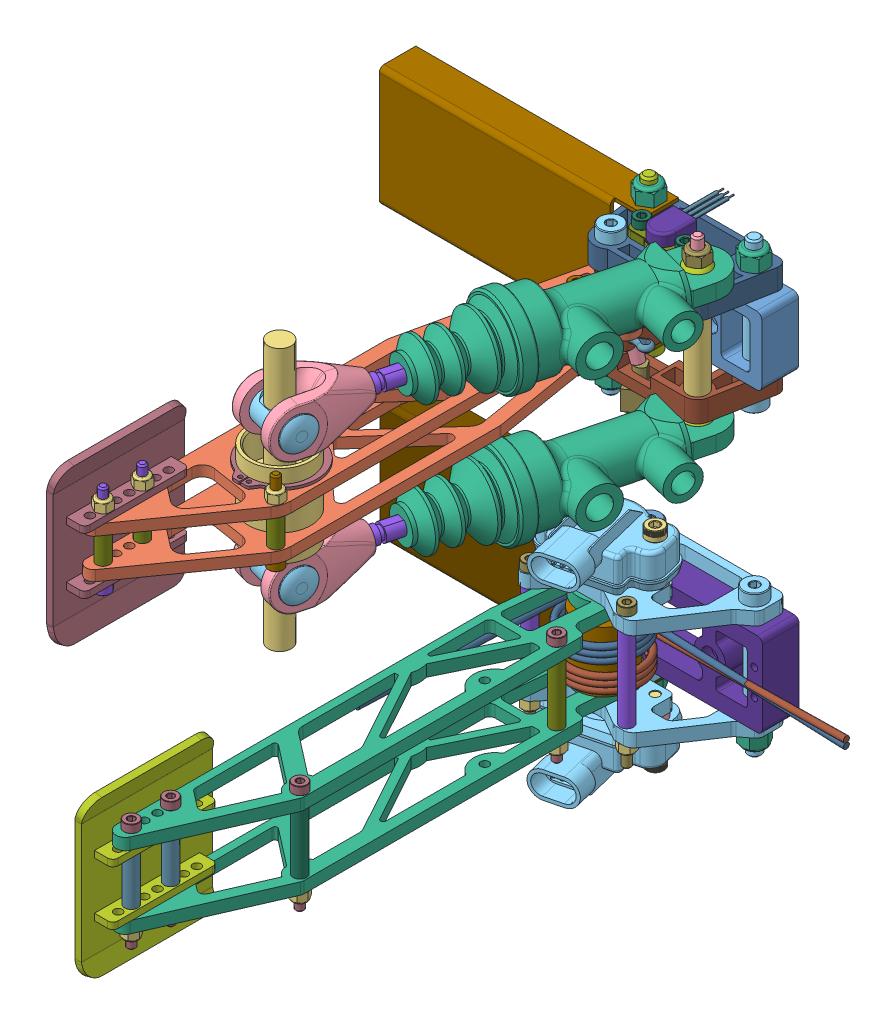
SolidWorks assembly BR-A10001-BC-Pedal Box Assembly, configuration Default. Lengths in mm.
Overall size (234.39 254.99 284.61).
117 component instances, 60 part files, 3 mates.
Components (placement in the parent):
- BR-10001-DC-Brake Pedal Assembly-1: BR-10001-DC-Brake Pedal Assembly [Default] at (189.4552 74.6925 66.1604) size (203.2 127 284.61)
  - BR-X000X-BC-Brake Pedal Platform-1: BR-X000X-BC-Brake Pedal Platform [Default] at (101.6 16.51 0) size (203.2 33.02 17.78)
  - BR-20002-AG-Brake Pedal Arm-3: BR-20002-AG-Brake Pedal Arm [Topo] at (131.445 12.065 13.97) size (50.8 6.35 239.54)
  - BR-20002-AG-Brake Pedal Arm-4: BR-20002-AG-Brake Pedal Arm [Topo] at (131.445 -6.985 13.97) size (50.8 6.35 239.54)
  - BR-00005-AA-Balance Bar (Tilton 600 Series)-1: BR-00005-AA-Balance Bar (Tilton 600 Series) [Default] at (131.445 0 174.2165) x (0.970657 0 0.240469) z (-0.240469 0 0.970657) size (31.09 127 49.61)
    - Copy of Bar^BR-00005-AA-Balance Bar (Tilton 600 Series)-1: Copy of Bar^BR-00005-AA-Balance Bar (Tilton 600 Series) [Default] at origin size (30.18 127 30.18) (virtual)
    - BB Arm^BR-00005-AA-Balance Bar (Tilton 600 Series)-1: BB Arm^BR-00005-AA-Balance Bar (Tilton 600 Series) [Default] at (-0.1778 -63.792 -0.0023) x (0 -1 0) z (-0.999904 0 -0.013855) size (32.63 46.01 30.45) (virtual)
    - BB Bullet^BR-00005-AA-Balance Bar (Tilton 600 Series)-3: BB Bullet^BR-00005-AA-Balance Bar (Tilton 600 Series) [Default] at (0 0.2208 0) x (0 1 0) z (0.999927 0 0.012056) size (15.81 15.82 29.99) (virtual)
    - BB Bullet^BR-00005-AA-Balance Bar (Tilton 600 Series)-4: BB Bullet^BR-00005-AA-Balance Bar (Tilton 600 Series) [Default] at (0 -0.2208 0) x (0 -1 0) z (0.999904 0 0.013855) size (15.81 15.82 29.99) (virtual)
    - BB Arm^BR-00005-AA-Balance Bar (Tilton 600 Series)-2: BB Arm^BR-00005-AA-Balance Bar (Tilton 600 Series) [Default] at (-0.1778 -0.2208 -0.0023) x (0 -1 0) z (-0.999904 0 -0.013855) size (32.63 46.01 30.45) (virtual)
  - BR-00004-AB-CP7855 Master Cylinder-1: BR-00004-AB-CP7855 Master Cylinder [14mm (0.55") Bore (88PRTE)] at (173.355 31.7856 13.97) x (-0.253024 0 0.96746) z (0.96746 0 0.253024) size (168.09 39 46.5) (flexible)
    - Main Body^BR-00004-AB-CP7855 Master Cylinder-1: Main Body^BR-00004-AB-CP7855 Master Cylinder [14.0-19.1mm (0.55"-0.75") Bore] x (0 0 1) z (1 0 0) size (46.5 39 130) (virtual)
    - Spherical Mount^BR-00004-AB-CP7855 Master Cylinder-1: Spherical Mount^BR-00004-AB-CP7855 Master Cylinder [Default] at origin size (14 11.1 14) (virtual)
    - Threaded Piston^BR-00004-AB-CP7855 Master Cylinder-1: Threaded Piston^BR-00004-AB-CP7855 Master Cylinder [Default] at (95.5875 0 0) size (60 8 8) (virtual)
  - BR-00004-AB-CP7855 Master Cylinder-2: BR-00004-AB-CP7855 Master Cylinder [14mm (0.55") Bore (88PRTE)] at (173.355 -31.7856 13.97) x (-0.253024 0 0.96746) z (0.96746 0 0.253024) size (168.09 39 46.5) (flexible)
    - Main Body^BR-00004-AB-CP7855 Master Cylinder-1: Main Body^BR-00004-AB-CP7855 Master Cylinder [14.0-19.1mm (0.55"-0.75") Bore] x (0 0 1) z (1 0 0) size (46.5 39 130) (virtual)
    - Spherical Mount^BR-00004-AB-CP7855 Master Cylinder-1: Spherical Mount^BR-00004-AB-CP7855 Master Cylinder [Default] at origin size (14 11.1 14) (virtual)
    - Threaded Piston^BR-00004-AB-CP7855 Master Cylinder-1: Threaded Piston^BR-00004-AB-CP7855 Master Cylinder [Default] at (95.5875 0 0) size (60 8 8) (virtual)
  - BR-00001-BC-Heel Plate-1: BR-00001-BC-Heel Plate [Default] at (70.485 0 1.5875) size (127 57.99 17.7)
  - BR-10001-BE-Brake Pedal Mount (Left)-5: BR-10001-BE-Brake Pedal Mount (Left) [Topo] at (131.445 16.51 13.97) size (65.9 10.16 41.91)
  - BR-10001-BF-Brake Pedal Mount (Right)-5: BR-10001-BF-Brake Pedal Mount (Right) [Topo] at (131.445 -26.67 13.97) size (66.67 20.32 39.69)
  - FR-00006-AA-BOTS M2011SD3W01-1: FR-00006-AA-BOTS M2011SD3W01 [Default] at (146.05 -28.1686 13.97) x (0.819152 0 -0.573576) z (0 1 0) size (13 10.01 34.12)
  - BR-30003-BF-Toe Plate-2: BR-30003-BF-Toe Plate [Default] at (106.045 0 226.695) x (1 0 0) z (0 0 -1) size (12.06 76.34 63.5)
  - BR-00009-DA-BPPS (MSC360-1A-C0004-ERA360-05K)-1: BR-00009-DA-BPPS (MSC360-1A-C0004-ERA360-05K) [Default] at (148.209 35.87 5.334) x (1 0 0) z (0 -1 0) size (28 38 12.8)
    - MSC-360^BR-00009-DA-BPPS (MSC360-1A-C0004-ERA360-05K)-1: MSC-360^BR-00009-DA-BPPS (MSC360-1A-C0004-ERA360-05K) [Default] at origin size (28 38 12.8) (virtual)
      - 3981_subjto PCB^MSC-360_BR-00009-DA-BPPS (MSC360-1A-C0004-ERA360-05K)-1: 3981_subjto PCB^MSC-360_BR-00009-DA-BPPS (MSC360-1A-C0004-ERA360-05K) [Default] at (0 0 7.7) x (-1 0 0) z (0 0 -1) size (6.58 26 1.58) (virtual)
        - 3980_cable^3981_subjto PCB_MSC-360_BR-00009-DA-BPPS (MSC360-1A-C0004-ERA360-05K)-1: 3980_cable^3981_subjto PCB_MSC-360_BR-00009-DA-BPPS (MSC360-1A-C0004-ERA360-05K) [Default] at (0 -8.5 5.3) x (-1 0 0) z (0 -1 0) size (1.58 1.58 26) (virtual)
        - 3980_cable^3981_subjto PCB_MSC-360_BR-00009-DA-BPPS (MSC360-1A-C0004-ERA360-05K)-2: 3980_cable^3981_subjto PCB_MSC-360_BR-00009-DA-BPPS (MSC360-1A-C0004-ERA360-05K) [Default] at (2.5 -8.5 5.3) x (-1 0 0) z (0 -1 0) size (1.58 1.58 26) (virtual)
        - 3980_cable^3981_subjto PCB_MSC-360_BR-00009-DA-BPPS (MSC360-1A-C0004-ERA360-05K)-3: 3980_cable^3981_subjto PCB_MSC-360_BR-00009-DA-BPPS (MSC360-1A-C0004-ERA360-05K) [Default] at (-2.5 -8.5 5.3) x (-1 0 0) z (0 -1 0) size (1.58 1.58 26) (virtual)
      - 3987 rotor sobremoldeo^MSC-360_BR-00009-DA-BPPS (MSC360-1A-C0004-ERA360-05K)-1: 3987 rotor sobremoldeo^MSC-360_BR-00009-DA-BPPS (MSC360-1A-C0004-ERA360-05K) [Default] at (0 0 7.7) x (-1 0 0) z (0 0 1) size (1.9 5.9 3) (virtual)
        - 3987_rotor sobremoldeado^3987 rotor sobremoldeo_MSC-360_BR-00009-DA-BPPS (MSC360-1A-C0004-ERA360-05K)-1: 3987_rotor sobremoldeado^3987 rotor sobremoldeo_MSC-360_BR-00009-DA-BPPS (MSC360-1A-C0004-ERA360-05K) [Default] at origin size (1.9 5.9 3) (virtual)
      - 4048_carcasa MSC-360-G01-001^MSC-360_BR-00009-DA-BPPS (MSC360-1A-C0004-ERA360-05K)-1: 4048_carcasa MSC-360-G01-001^MSC-360_BR-00009-DA-BPPS (MSC360-1A-C0004-ERA360-05K) [Default] at origin size (28 16.5 9.5) (virtual)
      - 3982_apantallamiento^MSC-360_BR-00009-DA-BPPS (MSC360-1A-C0004-ERA360-05K)-1: 3982_apantallamiento^MSC-360_BR-00009-DA-BPPS (MSC360-1A-C0004-ERA360-05K) [Default] at origin size (12 16 7.5) (virtual)
  - BR-00012-AA-BPPS Linkage Barrel-2: BR-00012-AA-BPPS Linkage Barrel [Default] at (148.209 26.07 5.334) x (0 0 1) z (-1 0 0) size (9.53 19.05 9.53)
  - BR-00010-AC-BPPS Linkage A-1: BR-00010-AC-BPPS Linkage A [Default] at (148.209 3.845 5.334) size (12.7 3.17 29.59)
  - BR-00011-AC-BPPS Linkage B-1: BR-00011-AC-BPPS Linkage B [Default] at (131.445 0.67 30.48) x (0.766423 0 -0.642336) z (0.642336 0 0.766423) size (27.3 3.17 16.64)
  - BR-Steel Nylon Locknut, Grade 8, M4x0.7 (90576A103)-2: BR-Steel Nylon Locknut, Grade 8, M4x0.7 (90576A103) [90576A103] at (131.445 -14.565 30.48) x (0.429902 0 -0.902875) z (0 -1 0) size (7 8.08 5)
  - BR-Alloy Steel Shoulder B18.3 SHCS,  0.25x10-24, 3 in Lg (91259A106)-1: BR-Alloy Steel Shoulder B18.3 SHCS,  0.25x10-24, 3 in Lg (91259A106) [90298A552] at (173.355 3.1456 13.97) x (-0.999987 0 -0.005104) z (0 -1 0) size (9.53 9.53 90.67)
  - BR-Alloy Steel Shoulder B18.3 SHCS,  0.3125x0.25-20, 2.125 in Lg  (91259A480)-2: BR-Alloy Steel Shoulder B18.3 SHCS,  0.3125x0.25-20, 2.125 in Lg  (91259A480) [91259A480] at (131.445 32.2263 13.97) x (-0.837169 0 -0.546944) z (0 1 0) size (11.11 11.11 70.87)
  - BR-Steel Nylon Locknut, Grade 8, 0.25-20 (90630A110)-2: BR-Steel Nylon Locknut, Grade 8, 0.25-20 (90630A110) [90630A110] at (131.445 -26.67 13.97) x (-0.311254 0 -0.950327) z (-0.950327 0 0.311254) size (11.11 7.94 12.83)
  - BR-Alloy Steel Shoulder B18.3 SHCS,  0.3125x0.25-20, 2.25 in (91259A108)-3: BR-Alloy Steel Shoulder B18.3 SHCS,  0.3125x0.25-20, 2.25 in (91259A108) [91259A108] at (127 2.359 -8.89) x (-1 0 0) z (0 -1 0) size (11.11 11.11 74.05)
  - BR-Alloy Steel Shoulder B18.3 SHCS,  0.3125x0.25-20, 2.125 in Lg  (91259A480)-4: BR-Alloy Steel Shoulder B18.3 SHCS,  0.3125x0.25-20, 2.125 in Lg  (91259A480) [91259A480] at (177.8 -32.2263 -8.89) x (1 0 0) z (0 -1 0) size (11.11 11.11 70.87)
  - BR-Steel Nylon Locknut, Grade 8, 0.25-20 (90630A110)-3: BR-Steel Nylon Locknut, Grade 8, 0.25-20 (90630A110) [90630A110] at (177.8 26.67 -8.89) size (11.11 7.94 12.83)
  - BR-Steel Nylon Locknut, Grade 8, 0.25-20 (90630A110)-4: BR-Steel Nylon Locknut, Grade 8, 0.25-20 (90630A110) [90630A110] at (127 28.5242 -8.89) size (11.11 7.94 12.83)
  - BR-Steel Nylon Locknut, Grade 8, M4x0.7 (90576A103)-3: BR-Steel Nylon Locknut, Grade 8, M4x0.7 (90576A103) [90576A103] at (146.05 14.565 190.7265) x (1 0 0) z (0 1 0) size (7 8.08 5)
  - FS-BLACK OXIDE C12.9 SHCS, M4x0.7-40 (91290A184)-12: FS-BLACK OXIDE C12.9 SHCS, M4x0.7-40 (91290A184) [91290A184] at (111.125 2.76 239.395) x (-1 0 0) z (0 -1 0) size (7 7 44.17)
  - BR-Steel Nylon Locknut, Grade 8, M4x0.7 (90576A103)-4: BR-Steel Nylon Locknut, Grade 8, M4x0.7 (90576A103) [90576A103] at (111.125 17.74 239.395) x (-1 0 0) z (0 1 0) size (7 8.08 5)
  - FS-BLACK OXIDE C12.9 SHCS, M4x0.7-40 (91290A184)-13: FS-BLACK OXIDE C12.9 SHCS, M4x0.7-40 (91290A184) [91290A184] at (111.125 2.76 220.345) x (1 0 0) z (0 -1 0) size (7 7 44.17)
  - BR-Steel Nylon Locknut, Grade 8, M4x0.7 (90576A103)-5: BR-Steel Nylon Locknut, Grade 8, M4x0.7 (90576A103) [90576A103] at (111.125 17.74 220.345) x (1 0 0) z (0 1 0) size (7 8.08 5)
  - BR-Black Oxide C12.9 SHCS, M4x0.7-35 (91290A173)-10: BR-Black Oxide C12.9 SHCS, M4x0.7-35 (91290A173) [91290A173] at (146.05 3.435 190.7265) x (1 0 0) z (0 -1 0) size (7 7 39.17)
  - BR-Black Oxide C12.9 SHCS, M4x0.7-12 (91290A148)-3: BR-Black Oxide C12.9 SHCS, M4x0.7-12 (91290A148) [91290A148] at (148.209 7.845 5.334) x (1 0 0) z (0 -1 0) size (7 7 16.17)
  - BR-Black Oxide C12.9 SHCS, M4x0.7-35 (91290A173)-11: BR-Black Oxide C12.9 SHCS, M4x0.7-35 (91290A173) [91290A173] at (131.445 -3.435 30.48) x (0.827693 0 0.561181) z (0 1 0) size (7 7 39.17)
  - BR-Steel Nylon Locknut, Grade 8, M4x0.7 (90576A103)-8: BR-Steel Nylon Locknut, Grade 8, M4x0.7 (90576A103) [90576A103] at (158.709 14.01 5.334) x (1 0 0) z (0 -1 0) size (7 8.08 5)
  - 1004-1045 Carbon Steel Clevis Pin (98306A210)-1: 1004-1045 Carbon Steel Clevis Pin (98306A210) [98306A210] at (148.209 0.67 24.384) x (0.997566 0 -0.069732) z (0 1 0) size (11.18 11.18 15.24)
  - BR-Stainless Steel Nylon Locknut, 10-24 (91831A011)-1: BR-Stainless Steel Nylon Locknut, 10-24 (91831A011) [91831A011] at (173.355 37.3356 13.97) size (9.53 6.11 11)
  - BR-Spring Steel External Retaining Ring, 1.176 ID (97633A340)-3: BR-Spring Steel External Retaining Ring, 1.176 ID (97633A340) [97633A340] at (131.445 -12.7 174.2165) x (0 1 0) z (1 0 0) size (1.27 37.56 34.79)
  - BR-Spring Steel External Retaining Ring, 1.176 ID (97633A340)-4: BR-Spring Steel External Retaining Ring, 1.176 ID (97633A340) [97633A340] at (131.445 12.7 174.2165) x (0 1 0) z (1 0 0) size (1.27 37.56 34.79)
  - BR-Zinc-Plated 1004-1045 Carbon Steel Cotter Pins, 0.5 Lg (98338A170)-1: BR-Zinc-Plated 1004-1045 Carbon Steel Cotter Pins, 0.5 Lg (98338A170) [98338A170] at (140.5409 -1.1159 24.92) x (-0.997566 0 0.069732) z (0 -1 0) size (22.21 6.3 3.05)
  - 91290A168_Alloy Steel Socket Head Screw M4x0.7,20-1: 91290A168_Alloy Steel Socket Head Screw M4x0.7,20 [91290A168] at (158.709 22.17 5.334) x (1 0 0) z (0 1 0) size (7 7 24.04)
  - BR-0000X-AC-Toe Plate Spacer-1: BR-0000X-AC-Toe Plate Spacer [Default] at (111.125 6.985 239.395) size (6.35 13.97 6.35)
  - BR-0000X-AC-Toe Plate Spacer-2: BR-0000X-AC-Toe Plate Spacer [Default] at (111.125 6.985 220.345) size (6.35 13.97 6.35)
  - BR-0000X-AC-Toe Plate Spacer-3: BR-0000X-AC-Toe Plate Spacer [Default] at (146.05 6.985 190.7265) size (6.35 13.97 6.35)
  - BR-0000X-AC-Brake Pedal Arm Spacer, Mid-1: BR-0000X-AC-Brake Pedal Arm Spacer, Mid [Default] at (131.445 6.985 13.97) size (11.11 13.97 11.11)
  - BR-0000X-AC-Brake Pedal Arm Spacer, Sides-1: BR-0000X-AC-Brake Pedal Arm Spacer, Sides [Default] at (131.445 16.51 13.97) size (11.11 4.45 11.11)
  - BR-0000X-AC-Brake Pedal Arm Spacer, Sides-2: BR-0000X-AC-Brake Pedal Arm Spacer, Sides [Default] at (131.445 -12.065 13.97) size (11.11 4.45 11.11)
  - BR-0000X-AA-BPPS Spacer, Long-1: BR-0000X-AA-BPPS Spacer, Long [Default] at (131.445 0.635 30.48) size (7 7.62 7)
  - BR-0000X-AA-BPPS Spacer, Short-1: BR-0000X-AA-BPPS Spacer, Short [Default] at (131.445 6.985 30.48) size (6.35 3.05 6.35)
  - BR-0000X-AB-Brake Mount Spacer-1: BR-0000X-AB-Brake Mount Spacer [Default] at (173.355 16.51 13.97) size (9.53 33.02 9.53)
  - 91290A168_Alloy Steel Socket Head Screw M4x0.7,20-2: 91290A168_Alloy Steel Socket Head Screw M4x0.7,20 [91290A168] at (137.709 22.17 5.334) x (1 0 0) z (0 1 0) size (7 7 24.04)
  - BR-Steel Nylon Locknut, Grade 8, M4x0.7 (90576A103)-9: BR-Steel Nylon Locknut, Grade 8, M4x0.7 (90576A103) [90576A103] at (137.709 14.01 5.334) x (-1 0 0) z (0 -1 0) size (7 8.08 5)
  - FR-0000X-AA-BOTS CAP-1: FR-0000X-AA-BOTS CAP [Default] at (145.1905 -18.4439 14.5719) x (0.89662 0.212244 -0.388618) z (-0.177297 0.976296 0.124145) size (5.59 5.59 11.05)
- BR-10001-CE-Accel Pedal Assembly-1: BR-10001-CE-Accel Pedal Assembly [Default] at (481.8727 -65.0075 66.1604) size (227.08 103.57 268.92)
  - BR-1000X-CD-Accel Pedal Mount-1: BR-1000X-CD-Accel Pedal Mount [Model] at (-163.5125 -20.32 13.0175) size (80.67 6.35 54.51)
  - BR-1000X-CD-Accel Pedal Mount-2: BR-1000X-CD-Accel Pedal Mount [Model] at (-163.5125 26.67 13.0175) size (80.67 6.35 54.51)
  - BR-2000X-BD-Accel_Pedal_Arm-3: BR-2000X-BD-Accel_Pedal_Arm [Default] at (-163.5125 14.732 13.0175) size (33.81 6.35 244.97)
  - BR-2000X-BD-Accel_Pedal_Arm-4: BR-2000X-BD-Accel_Pedal_Arm [Default] at (-163.5125 -20.32 13.0175) size (33.81 6.35 244.97)
  - BR-30003-BE-Accel Toe Plate-1: BR-30003-BE-Accel Toe Plate [Default] at (-180.0225 0 219.3925) x (1 0 0) z (0 0 -1) size (12.06 76.42 63.5)
  - BR-0000X-AA-AP Mount Spacer-1: BR-0000X-AA-AP Mount Spacer [Default] at (-139.5 20.32 27.7211) size (6.35 40.64 6.35)
  - BR-X000X-BC-Torsion Spring Shaft-1: BR-X000X-BC-Torsion Spring Shaft [Default] at (-159.8809 14.478 18.6236) x (0.999483 0 0.032158) z (-0.032158 0 0.999483) size (26.19 29.21 26.19)
  - BR-AD-Torsion Spring (9271K663)-1: BR-AD-Torsion Spring (9271K663) [9271K663] at (-159.8809 10.9639 18.6236) x (0 -1 0) z (-0.011992 0 0.999928) size (18.11 120.03 122.87)
  - BR-AD-Torsion Spring, Left Wound (9271K597)-1: BR-AD-Torsion Spring, Left Wound (9271K597) [9271K597] at (-159.8809 -1.547 18.6236) x (0 -1 0) z (-0.011992 0 0.999928) size (18.11 122.87 120.03)
  - BR-Steel Nylon Locknut, Grade 8, M4x0.7 (90576A103)-1: BR-Steel Nylon Locknut, Grade 8, M4x0.7 (90576A103) [90576A103] at (-150.0266 -22.82 51.1175) x (1 0 0) z (0 -1 0) size (7 8.08 5)
  - BR-Alloy Steel Shoulder B18.3 SHCS,  0.3125x0.25-20, 2.125 in Lg  (91259A480)-2: BR-Alloy Steel Shoulder B18.3 SHCS,  0.3125x0.25-20, 2.125 in Lg  (91259A480) [91259A480] at (-114.3 32.2263 -8.89) x (0 0 1) z (0 1 0) size (11.11 11.11 70.87)
  - BR-Black Oxide C12.9 SHCS, M4x0.7-65 (91290A083)-5: BR-Black Oxide C12.9 SHCS, M4x0.7-65 (91290A083) [91290A083] at (-181.2925 -3.83 32.9235) x (1 0 0) z (0 1 0) size (7 7 69.17)
  - BR-Black Oxide C12.9 SHCS, M4x0.7-65 (91290A083)-6: BR-Black Oxide C12.9 SHCS, M4x0.7-65 (91290A083) [91290A083] at (-139.5 -3.83 27.7211) x (1 0 0) z (0 1 0) size (7 7 69.17)
  - BR-Black Oxide C12.9 SHCS, M4x0.7-50 (91290A186)-1: BR-Black Oxide C12.9 SHCS, M4x0.7-50 (91290A186) [91290A186] at (-174.9425 -2.68 232.0925) x (1 0 0) z (0 1 0) size (7 7 54.17)
  - BR-Black Oxide C12.9 SHCS, M4x0.7-50 (91290A186)-2: BR-Black Oxide C12.9 SHCS, M4x0.7-50 (91290A186) [91290A186] at (-174.9425 -2.68 213.0425) x (1 0 0) z (0 1 0) size (7 7 54.17)
  - BR-Black Oxide C12.9 SHCS, M4x0.7-50 (91290A186)-3: BR-Black Oxide C12.9 SHCS, M4x0.7-50 (91290A186) [91290A186] at (-150.0266 -2.68 175.4283) x (1 0 0) z (0 1 0) size (7 7 54.17)
  - BR-Steel Nylon Locknut, Grade 8, M4x0.7 (90576A103)-4: BR-Steel Nylon Locknut, Grade 8, M4x0.7 (90576A103) [90576A103] at (-174.9425 -22.82 232.0925) x (0 0 1) z (0 -1 0) size (7 8.08 5)
  - BR-Steel Nylon Locknut, Grade 8, M4x0.7 (90576A103)-5: BR-Steel Nylon Locknut, Grade 8, M4x0.7 (90576A103) [90576A103] at (-174.9425 -22.82 213.0425) x (0 0 1) z (0 -1 0) size (7 8.08 5)
  - BR-Steel Nylon Locknut, Grade 8, M4x0.7 (90576A103)-6: BR-Steel Nylon Locknut, Grade 8, M4x0.7 (90576A103) [90576A103] at (-150.0266 -22.82 175.4283) x (0 0 1) z (0 -1 0) size (7 8.08 5)
  - BR-Steel Nylon Locknut, Grade 8, M4x0.7 (90576A103)-7: BR-Steel Nylon Locknut, Grade 8, M4x0.7 (90576A103) [90576A103] at (-181.2925 -29.17 32.9235) x (0.973511 0 0.228641) z (0 -1 0) size (7 8.08 5)
  - BR-Steel Nylon Locknut, Grade 8, M4x0.7 (90576A103)-8: BR-Steel Nylon Locknut, Grade 8, M4x0.7 (90576A103) [90576A103] at (-139.5 -29.17 27.7211) x (1 0 0) z (0 -1 0) size (7 8.08 5)
  - BR-Steel Nylon Locknut, Grade 8, 0.25-20 (90630A110)-1: BR-Steel Nylon Locknut, Grade 8, 0.25-20 (90630A110) [90630A110] at (-114.3 -26.67 -8.89) x (0 0 1) z (1 0 0) size (11.11 7.94 12.83)
  - BR-Steel Nylon Locknut, Grade 8, 0.25-20 (90630A110)-2: BR-Steel Nylon Locknut, Grade 8, 0.25-20 (90630A110) [90630A110] at (-165.1 -28.9941 -8.89) x (0 0 1) z (1 0 0) size (11.11 7.94 12.83)
  - BR-0000X-AA-AP Mount Spacer-4: BR-0000X-AA-AP Mount Spacer [Default] at (-181.2925 20.32 32.9235) size (6.35 40.64 6.35)
  - BR-0000X-AA-AP Toe Plate Spacer-1: BR-0000X-AA-AP Toe Plate Spacer [Default] at (-174.9425 11.557 232.0925) size (6.35 23.11 6.35)
  - BR-0000X-AA-AP Toe Plate Spacer-2: BR-0000X-AA-AP Toe Plate Spacer [Default] at (-174.9425 11.557 213.0425) size (6.35 23.11 6.35)
  - BR-0000X-AA-AP Arm Spacer-1: BR-0000X-AA-AP Arm Spacer [Default] at (-150.0266 14.732 175.4283) size (6.35 29.46 6.35)
  - BR-0000X-AA-APPS Spacer, Right-1: BR-0000X-AA-APPS Spacer, Right [Default] at (-150.0266 14.732 51.1175) size (6.35 29.46 6.35)
  - BR-0000X-CC-Accel Pedal Platform-1: BR-0000X-CC-Accel Pedal Platform [Default] at (-92.8688 0 0) size (195.26 40.64 17.78)
  - BR-00001-BD-Heel Plate-2: BR-00001-BD-Heel Plate [Default] at (-221.615 0 1.5875) size (127 57.99 17.7)
  - BR-Alloy Steel Shoulder B18.3 SHCS,  0.3125x0.25-20, 2.25 in Lg  (91259A108)-1: BR-Alloy Steel Shoulder B18.3 SHCS,  0.3125x0.25-20, 2.25 in Lg  (91259A108) [91259A108] at (-165.1 -2.359 -8.89) x (-0.837169 0 -0.546944) z (0 1 0) size (11.11 11.11 74.05)
  - BR-Black Oxide C12.9 SHCS, M4x0.7-50 (91290A186)-4: BR-Black Oxide C12.9 SHCS, M4x0.7-50 (91290A186) [91290A186] at (-150.0266 -2.68 51.1175) x (-0.837169 0 -0.546944) z (0 1 0) size (7 7 54.17)
  - BR-00002-AA 2868T4_High-Load Oil-Embedded 863 Sleeve Bearing 0.375 in ID-2: BR-00002-AA 2868T4_High-Load Oil-Embedded 863 Sleeve Bearing 0.375 in ID [2868T4] at (-163.5125 23.495 13.0175) x (1 0 0) z (0 -1 0) size (12.75 12.75 6.35)
  - BR-00002-AA 2868T4_High-Load Oil-Embedded 863 Sleeve Bearing 0.375 in ID-3: BR-00002-AA 2868T4_High-Load Oil-Embedded 863 Sleeve Bearing 0.375 in ID [2868T4] at (-163.5125 -23.495 13.0175) x (1 0 0) z (0 -1 0) size (12.75 12.75 6.35)
  - BR-90128A249_Zinc-Plated Alloy Steel Socket Head Screw M5x0.8-25-1: BR-90128A249_Zinc-Plated Alloy Steel Socket Head Screw M5x0.8-25 [90128A249] at (-181.9542 -35.6757 17.5895) x (1 0 0) z (0 -1 0) size (8.51 8.51 30.66)
  - BR-93657A069_Nylon Unthreaded Spacer 5.3mm ID 10mm OD-1: BR-93657A069_Nylon Unthreaded Spacer 5.3mm ID 10mm OD [93657A069] at (-181.9542 -28.17 17.5895) x (1 0 0) z (0 -1 0) size (10 10 3)
  - BR-9851R5KL2.0 Potentiometer Sensor-1: BR-9851R5KL2.0 Potentiometer Sensor [Default] at (-163.4903 -29.6045 13.1069) x (0.970617 0 -0.240632) z (0 -1 0) size (52.67 51.68 25.12)
  - BR-9851R5KL2.0 Potentiometer Sensor-2: BR-9851R5KL2.0 Potentiometer Sensor [Default] at (-163.4903 29.6045 13.1069) x (-0.970617 0 0.240632) z (0 1 0) size (52.67 51.68 25.12)
  - BR-90128A249_Zinc-Plated Alloy Steel Socket Head Screw M5x0.8-25-2: BR-90128A249_Zinc-Plated Alloy Steel Socket Head Screw M5x0.8-25 [90128A249] at (-181.9542 35.6757 17.5895) x (1 0 0) z (0 1 0) size (8.51 8.51 30.66)
  - BR-93657A069_Nylon Unthreaded Spacer 5.3mm ID 10mm OD-2: BR-93657A069_Nylon Unthreaded Spacer 5.3mm ID 10mm OD [93657A069] at (-145.0708 28.17 8.4455) x (1 0 0) z (0 -1 0) size (10 10 3)
  - BR-93657A069_Nylon Unthreaded Spacer 5.3mm ID 10mm OD-3: BR-93657A069_Nylon Unthreaded Spacer 5.3mm ID 10mm OD [93657A069] at (-181.9542 28.17 17.5895) x (1 0 0) z (0 -1 0) size (10 10 3)
  - BR-93657A069_Nylon Unthreaded Spacer 5.3mm ID 10mm OD-4: BR-93657A069_Nylon Unthreaded Spacer 5.3mm ID 10mm OD [93657A069] at (-145.0708 -28.17 8.4455) x (1 0 0) z (0 -1 0) size (10 10 3)
  - BR-90128A249_Zinc-Plated Alloy Steel Socket Head Screw M5x0.8-25-3: BR-90128A249_Zinc-Plated Alloy Steel Socket Head Screw M5x0.8-25 [90128A249] at (-145.0708 -35.6757 8.4455) x (0.970617 0 -0.240632) z (0 -1 0) size (8.51 8.51 30.66)
  - BR-90128A249_Zinc-Plated Alloy Steel Socket Head Screw M5x0.8-25-4: BR-90128A249_Zinc-Plated Alloy Steel Socket Head Screw M5x0.8-25 [90128A249] at (-145.0708 35.6757 8.4455) x (1 0 0) z (0 1 0) size (8.51 8.51 30.66)
  - BR-00001-BA D-Shaft-1: BR-00001-BA D-Shaft [Default] at (-163.5125 0 13.0175) x (-0.359671 0 0.933079) z (-0.933079 0 -0.359671) size (9.53 85 8.88)
Mates (geometry in assembly coordinates):
- Distance2: distance = 6.35 mm aligned: plane of BR-10001-DC-Brake Pedal Assembly-1/BR-30003-BF-Toe Plate-2 through (292.3252 44.2066 268.7194) normal (-1 0 0); plane of BR-10001-CD-Accel Pedal Assembly-1/BR-30003-BE-Accel Toe Plate-1 through (298.6752 -95.4934 261.4169) normal (-1 0 0)
- Coincident2: coincident aligned: plane of BR-10001-DC-Brake Pedal Assembly-1/BR-X000X-BC-Brake Pedal Platform-1 through (392.6552 58.1825 48.3804) normal (0 0 -1); plane of BR-10001-CD-Accel Pedal Assembly-1/BR-0000X-CC-Accel Pedal Platform-1 through (389.0039 -65.0075 48.3804) normal (0 0 -1)
- Distance1: distance = 102.87 mm anti-aligned: plane of BR-10001-DC-Brake Pedal Assembly-1/BR-X000X-BC-Brake Pedal Platform-1 through (291.0552 58.1825 66.1604) normal (0 -1 0); plane of BR-10001-CD-Accel Pedal Assembly-1/BR-0000X-CC-Accel Pedal Platform-1 through (295.3414 -44.6875 48.3804) normal (0 1 0)
